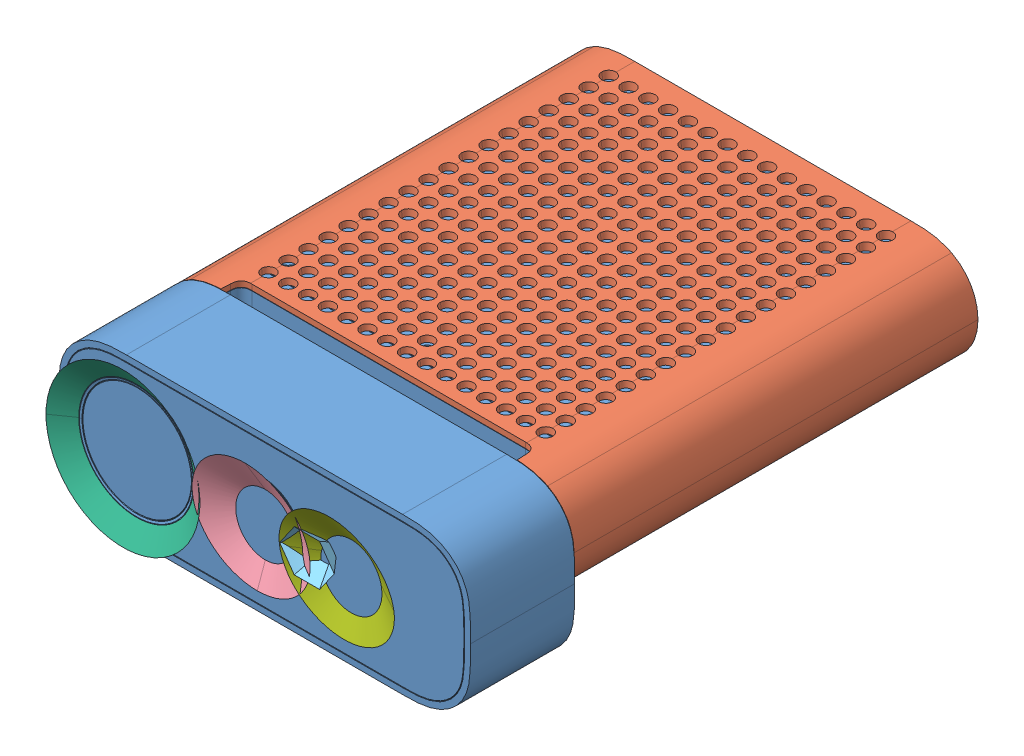
SolidWorks assembly akdk_camera_cad, configuration Default. Lengths in mm.
Overall size (103.01 39.05 132.52).
9 component instances, 7 part files, 0 mates.
Components (placement in the parent):
- akdk_camera_cad.stp-1: akdk_camera_cad.stp [Default] at origin size (103.01 39.05 132.52)
  - CAMERA-BODY.stp-1: CAMERA-BODY.stp [Default] at origin size (103.01 39.01 125.44)
  - HOLDER-COVER.stp-1: HOLDER-COVER.stp [Default] at origin size (102.54 26.09 101.55)
  - SCREW_F25X7_T8_1.stp-1: SCREW_F25X7_T8_1.stp [Default] at (38.5 6.5 -126.6) x (1 0 0) z (0 1 0) size (5 7.07 5)
  - SCREW_F25X7_T8_1.stp-2: SCREW_F25X7_T8_1.stp [Default] at (-38.5 6.5 -126.6) x (1 0 0) z (0 1 0) size (5 7.07 5)
  - DEPTH-CONE-WITH-SENSOR-POSITION.stp-1: DEPTH-CONE-WITH-SENSOR-POSITION.stp [Default] at origin size (29.36 29.93 10.04)
  - IR1.stp-1: IR1.stp [Default] at origin size (13.74 10.52 6.08)
  - RGB-CONE-WITH-SENSOR-POSITION.stp-1: RGB-CONE-WITH-SENSOR-POSITION.stp [Default] at origin size (38.47 38.47 13.47)
  - IR2.stp-1: IR2.stp [Default] at origin size (28.59 28.36 8.93)
